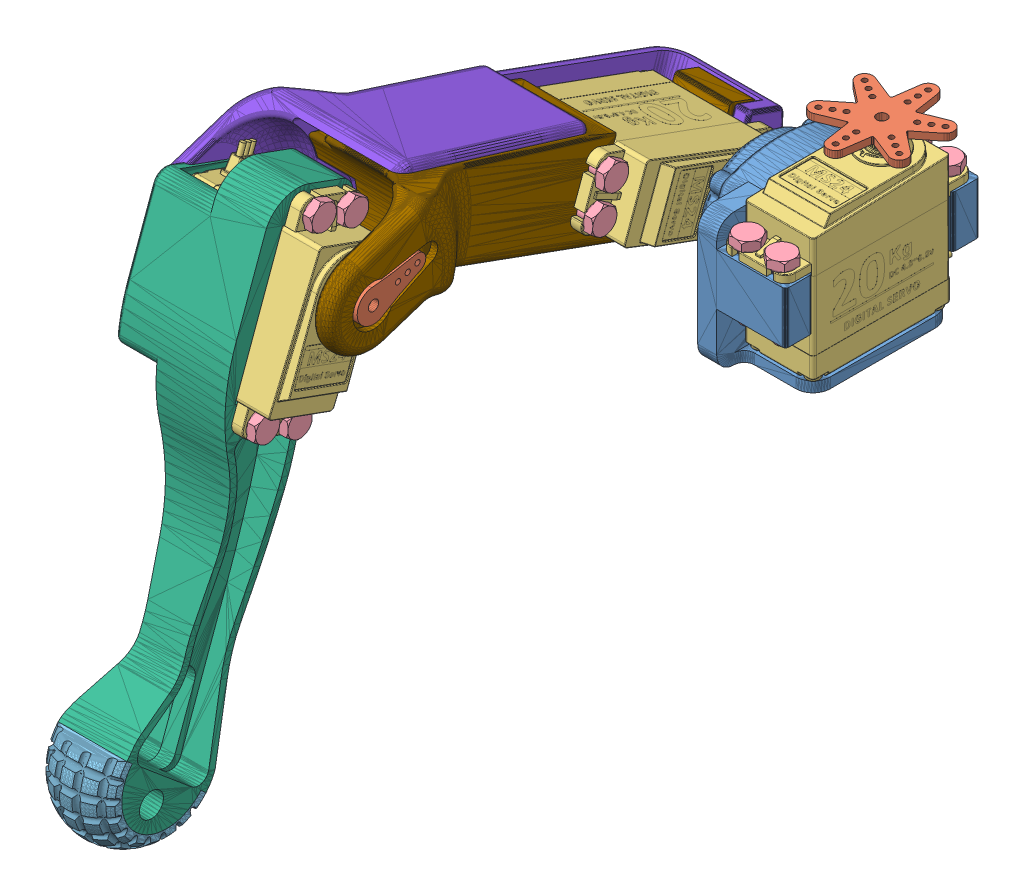
SolidWorks assembly Back Right Leg Assembly, configuration Default. Lengths in mm.
Overall size (104.56 167.25 200.75).
25 component instances, 9 part files, 60 mates.
Components (placement in the parent):
- Right_arm_joint_mg-1: Right_arm_joint_mg [Default] at (24.2858 18.5405 -25.0321) size (37.5 46 56.5)
- Servohorn-1: Servohorn [4 Prong] at (-38.4142 28.7905 -4.7821) x (0 0.715501 0.698611) z (-1 0 0) size (31.8 31.8 2.24)
- Servo Motor-1: Servo Motor [Default] at (-15.7142 38.5405 -14.5321) size (20.1 45.99 55.6)
- Servohorn-2: Servohorn [Default] at (-15.7142 58.9405 -14.5321) x (-0.99999 0 0.00451) z (0 -1 0) size (28.18 31.8 2.24)
- _Hex_Screws-1: _Hex_Screws [H M4x20] at (-20.7142 41.7405 19.4679) x (-0.837169 0 -0.546944) z (-0.546944 0 0.837169) size (7 22.8 8.08)
- _Hex_Screws-2: _Hex_Screws [H M4x20] at (-10.7142 41.7405 -28.5321) x (-0.837169 0 -0.546944) z (-0.546944 0 0.837169) size (7 22.8 8.08)
- _Hex_Screws-3: _Hex_Screws [H M4x20] at (-10.7142 41.7405 19.4679) x (-0.99108 0 -0.133267) z (-0.133267 0 0.99108) size (7 22.8 8.08)
- _Hex_Screws-4: _Hex_Screws [H M4x20] at (-20.7142 41.7405 -28.5321) x (0.837169 0 0.546944) z (0.546944 0 -0.837169) size (7 22.8 8.08)
- _Hex_Screws-20: _Hex_Screws [H M3x16] at (-83.7173 43.6223 71.0537) x (0.992954 0.04053 0.111356) z (-0.118503 0.33961 0.933071) size (5.5 18 6.35)
- _Hex_Screws-21: _Hex_Screws [H M4x20] at (-66.0142 67.1041 99.9555) x (0 0.149128 -0.988818) z (0 0.988818 0.149128) size (7 22.8 8.08)
- _Hex_Screws-22: _Hex_Screws [H M4x20] at (-66.0142 63.6839 90.5585) x (0 -0.837169 0.546944) z (0 -0.546944 -0.837169) size (7 22.8 8.08)
- _Hex_Screws-23: _Hex_Screws [H M4x20] at (-66.0142 21.9989 116.3724) x (0 -0.837169 0.546944) z (0 -0.546944 -0.837169) size (7 22.8 8.08)
- _Hex_Screws-24: _Hex_Screws [H M4x20] at (-66.0142 18.5787 106.9755) x (0 -0.837169 0.546944) z (0 -0.546944 -0.837169) size (7 22.8 8.08)
- _Hex_Screws-25: _Hex_Screws [H M4x20] at (-55.6142 28.7007 -19.6479) x (0 0.663788 -0.747921) z (0 0.747921 0.663788) size (7 22.8 8.08)
- _Hex_Screws-26: _Hex_Screws [H M4x20] at (-55.6142 19.3037 -16.2277) x (0 -0.857577 0.514355) z (0 -0.514355 -0.857577) size (7 22.8 8.08)
- _Hex_Screws-27: _Hex_Screws [H M4x20] at (-55.6142 45.1176 25.4573) x (0 -0.837169 0.546944) z (0 -0.546944 -0.837169) size (7 22.8 8.08)
- _Hex_Screws-28: _Hex_Screws [H M4x20] at (-55.6142 35.7207 28.8775) x (0 -0.837169 0.546944) z (0 -0.546944 -0.837169) size (7 22.8 8.08)
- Servo Motor-4: Servo Motor [Default] at (-69.2142 52.2383 100.0453) x (0 -0.34202 -0.939693) z (0 -0.939693 0.34202) size (20.1 45.99 55.6)
- foot-2: foot [Default] at (-69.2142 -56.7491 139.7664) x (0 -0.642788 -0.766044) z (0 0.766044 -0.642788) size (38.32 20 19.41)
- Left_wrist_mg-1: Left_wrist_mg [Default] at (-39.2142 58.2322 87.2751) x (0 -0.939693 0.34202) z (0 0.34202 0.939693) size (149.99 36.9 30)
- Servohorn-4: Servohorn [1 Prong] at (-48.8142 52.2383 100.0453) x (0 -0.947083 -0.320989) z (-1 0 0) size (9.55 20.65 2.24)
- F625ZZ Ball Bearing-2: F625ZZ Ball Bearing [Default] at (-99.0142 54.8139 92.2998) x (0 0.948801 0.315873) z (1 0 0) size (18 18 5)
- SM_Left_arm_cover-1: SM_Left_arm_cover [Default] at (-59.0142 8.2739 -16.9989) x (0 0.939693 -0.34202) z (0 0.34202 0.939693) size (41.16 45 143.55)
- Left_arm_mg-1: Left_arm_mg [Default] at (-58.8142 15.8365 -11.1347) x (0 0.939693 -0.34202) z (0 0.34202 0.939693) size (38.24 39.8 137.4)
- Servo Motor-5: Servo Motor [Default] at (-58.8142 28.7905 -4.7821) x (0 -0.939693 0.34202) z (0 0.34202 0.939693) size (20.1 45.99 55.6)
Mates (geometry in assembly coordinates):
- Coincident1: coincident anti-aligned: plane of Right_arm_joint_mg-1 through (-40.4142 18.5405 -25.0321) normal (1 0 0); plane of Servohorn-1 through (-40.4142 28.7905 -4.7821) normal (-1 0 0)
- Angle2: planar angle = 0.069813 rad anti-aligned: plane of Right_arm_joint_mg-1 through (24.2858 29.9404 -17.8834) normal (0 0.847204 0.531268); plane of Servohorn-1 through (-40.4142 21.752 -2.4794) normal (0 -0.808081 -0.589071)
- Coincident4: coincident: point of Right_arm_joint_mg-1; line of Servohorn-1 through (-38.4142 28.7905 -4.7821) axis (1 0 0)
- Coincident5: coincident anti-aligned: plane of Right_arm_joint_mg-1 through (-25.7142 18.5405 -25.0321) normal (1 0 0); plane of Servo Motor-1 through (-25.7142 49.5405 -23.5321) normal (-1 0 0)
- Coincident6: coincident anti-aligned: plane of Right_arm_joint_mg-1 through (24.2858 11.0405 -25.0321) normal (0 1 0); plane of Servo Motor-1 through (-15.7142 11.0405 -14.5321) normal (0 -1 0)
- Distance2: distance = 0 mm anti-aligned: plane of Servo Motor-1 through (-25.7142 18.5405 15.4679) normal (0 0 1); plane of Right_arm_joint_mg-1 through (24.2858 18.5405 15.4679) normal (0 0 -1)
- Concentric1: concentric anti-aligned: cylinder of Servo Motor-1 through (-15.7142 52.9405 -14.5321) axis (0 1 0) radius 1.25; line of Servohorn-2 through (-15.7142 58.9405 -14.5321) axis (0 -1 0)
- Coincident8: coincident anti-aligned: plane of Servo Motor-1 through (-15.7142 56.9405 -14.5321) normal (0 1 0); plane of Servohorn-2 through (-15.7142 56.9405 -14.5321) normal (0 -1 0)
- Concentric4: concentric aligned: cylinder of Servo Motor-1 through (-10.7142 32.1765 19.4679) axis (0 1 0) radius 2.25; cylinder of _Hex_Screws-3 through (-10.7142 21.7405 19.4679) axis (0 1 0) radius 2
- Coincident35: coincident anti-aligned: plane of Servo Motor-1 through (-15.7142 41.7405 -14.5321) normal (0 1 0); plane of _Hex_Screws-3 through (-10.7142 41.7405 19.4679) normal (0 -1 0)
- Concentric5: concentric aligned: cylinder of Servo Motor-1 through (-20.7142 32.1765 19.4679) axis (0 1 0) radius 2.25; cylinder of _Hex_Screws-1 through (-20.7142 21.7405 19.4679) axis (0 1 0) radius 2
- Coincident36: coincident aligned: plane of _Hex_Screws-1 through (-20.7142 44.5405 19.4679) normal (0 1 0); plane of _Hex_Screws-3 through (-10.7142 44.5405 19.4679) normal (0 1 0)
- Concentric6: concentric aligned: cylinder of Servo Motor-1 through (-20.7142 32.1765 -28.5321) axis (0 1 0) radius 2.25; cylinder of _Hex_Screws-4 through (-20.7142 21.7405 -28.5321) axis (0 1 0) radius 2
- Coincident37: coincident anti-aligned: plane of Servo Motor-1 through (-15.7142 41.7405 -14.5321) normal (0 1 0); plane of _Hex_Screws-4 through (-20.7142 41.7405 -28.5321) normal (0 -1 0)
- Concentric7: concentric aligned: cylinder of Servo Motor-1 through (-10.7142 32.1765 -28.5321) axis (0 1 0) radius 2.25; cylinder of _Hex_Screws-2 through (-10.7142 21.7405 -28.5321) axis (0 1 0) radius 2
- Coincident38: coincident anti-aligned: plane of Servo Motor-1 through (-15.7142 41.7405 -14.5321) normal (0 1 0); plane of _Hex_Screws-2 through (-10.7142 41.7405 -28.5321) normal (0 -1 0)
- Coincident50: coincident anti-aligned: plane of Left_arm_mg-1 through (-58.8142 15.8365 -11.1347) normal (1 0 0); plane of Servo Motor-5 through (-58.8142 29.5678 23.6678) normal (-1 0 0)
- Angle5: planar angle = 0.069813 rad aligned: line of Left_arm_mg-1 through (-48.8142 60.1418 84.6186) axis (0 -0.180422 0.983589); line of Servohorn-4 through (-48.8142 57.5916 94.928) axis (0 -0.111371 0.993779)
- Coincident51: coincident anti-aligned: plane of Servo Motor-4 through (-96.7142 65.1665 106.0348) normal (0 0.34202 0.939693); plane of Left_wrist_mg-1 through (-39.2142 65.0726 106.069) normal (0 -0.34202 -0.939693)
- Coincident52: coincident: point of foot-2; line of Left_wrist_mg-1 through (-89.2142 -66.7075 148.1228) axis (0 0.687865 0.725839)
- Coincident53: coincident anti-aligned: plane of SM_Left_arm_cover-1 through (-59.0142 38.9729 67.346) normal (0 -0.34202 -0.939693); plane of Left_arm_mg-1 through (-58.8142 43.7662 65.6014) normal (0 0.34202 0.939693)
- Coincident54: coincident anti-aligned: plane of Servo Motor-4 through (-50.8142 52.2383 100.0453) normal (1 0 0); plane of Servohorn-4 through (-50.8142 52.2383 100.0453) normal (-1 0 0)
- Coincident55: coincident aligned: plane of foot-2 through (-89.2142 -56.7491 139.7664) normal (-1 0 0); plane of Left_wrist_mg-1 through (-89.2142 58.2322 87.2751) normal (-1 0 0)
- Coincident56: coincident anti-aligned: plane of SM_Left_arm_cover-1 through (-59.0142 15.3535 -19.5757) normal (0 -0.939693 0.34202); plane of Left_arm_mg-1 through (-58.8142 18.1228 -11.9669) normal (0 0.939693 -0.34202)
- Concentric8: concentric aligned: cylinder of Servo Motor-4 through (-54.8142 52.2383 100.0453) axis (1 0 0) radius 1.25; line of Servohorn-4 through (-48.8142 52.2383 100.0453) axis (1 0 0)
- Concentric9: concentric aligned: cylinder of _Hex_Screws-28 through (-75.6142 35.7207 28.8775) axis (1 0 0) radius 2; cylinder of Servo Motor-5 through (-65.1781 35.7207 28.8775) axis (1 0 0) radius 2.25
- Coincident57: coincident anti-aligned: plane of Servohorn-4 through (-50.8142 52.2383 100.0453) normal (-1 0 0); plane of Left_arm_mg-1 through (-50.8142 15.8365 -11.1347) normal (1 0 0)
- Concentric10: concentric aligned: cylinder of _Hex_Screws-27 through (-75.6142 45.1176 25.4573) axis (1 0 0) radius 2; cylinder of Servo Motor-5 through (-65.1781 45.1176 25.4573) axis (1 0 0) radius 2.25
- Coincident58: coincident anti-aligned: plane of Servo Motor-4 through (-69.2142 23.7885 100.8226) normal (-1 0 0); plane of Left_wrist_mg-1 through (-69.2142 58.2322 87.2751) normal (1 0 0)
- Coincident59: coincident anti-aligned: plane of F625ZZ Ball Bearing-2 through (-100.0142 49.7599 107.4806) normal (-1 0 0); plane of SM_Left_arm_cover-1 through (-100.0142 8.2739 -16.9989) normal (1 0 0)
- Coincident60: coincident anti-aligned: plane of SM_Left_arm_cover-1 through (-63.8142 8.2739 -16.9989) normal (-1 0 0); plane of Left_arm_mg-1 through (-63.8142 15.8365 -11.1347) normal (1 0 0)
- Coincident61: coincident anti-aligned: plane of Left_arm_mg-1 through (-58.8142 15.8365 -11.1347) normal (0 0.939693 -0.34202); plane of Servo Motor-5 through (-47.8142 29.3121 25.8892) normal (0 -0.939693 0.34202)
- Coincident62: coincident anti-aligned: plane of Left_arm_mg-1 through (-58.8142 29.6884 26.9228) normal (0 -0.34202 -0.939693); plane of Servo Motor-5 through (-86.3142 48.5292 20.0653) normal (0 0.34202 0.939693)
- Coincident63: coincident aligned: line of Servohorn-4 through (-48.8142 52.2383 100.0453) axis (1 0 0); line of Left_arm_mg-1 through (-50.8142 52.2383 100.0453) axis (1 0 0)
- Coincident64: coincident anti-aligned: plane of foot-2 through (-69.2142 -56.7491 139.7664) normal (0 0.766044 -0.642788); plane of Left_wrist_mg-1 through (-39.2142 -35.0884 165.5805) normal (0 -0.766044 0.642788)
- Coincident65: coincident anti-aligned: plane of Servo Motor-4 through (-89.2142 65.0555 106.022) normal (0 0.939693 -0.34202); plane of Left_wrist_mg-1 through (-39.2142 58.2322 87.2751) normal (0 -0.939693 0.34202)
- Concentric11: concentric aligned: cylinder of _Hex_Screws-23 through (-86.0142 21.9989 116.3724) axis (1 0 0) radius 2; cylinder of Servo Motor-4 through (-75.5781 21.9989 116.3724) axis (1 0 0) radius 2.25
- Concentric12: concentric aligned: cylinder of _Hex_Screws-26 through (-75.6142 19.3037 -16.2277) axis (1 0 0) radius 2; cylinder of Servo Motor-5 through (-65.1781 19.3037 -16.2277) axis (1 0 0) radius 2.25
- Coincident66: coincident anti-aligned: plane of _Hex_Screws-24 through (-66.0142 18.5787 106.9755) normal (-1 0 0); plane of Servo Motor-4 through (-66.0142 52.2383 100.0453) normal (1 0 0)
- Concentric13: concentric aligned: cylinder of _Hex_Screws-24 through (-86.0142 18.5787 106.9755) axis (1 0 0) radius 2; cylinder of Servo Motor-4 through (-75.5781 18.5787 106.9755) axis (1 0 0) radius 2.25
- Coincident67: coincident anti-aligned: plane of _Hex_Screws-28 through (-55.6142 35.7207 28.8775) normal (-1 0 0); plane of Servo Motor-5 through (-55.6142 28.7905 -4.7821) normal (1 0 0)
- Coincident68: coincident anti-aligned: plane of _Hex_Screws-23 through (-66.0142 21.9989 116.3724) normal (-1 0 0); plane of Servo Motor-4 through (-66.0142 52.2383 100.0453) normal (1 0 0)
- Coincident69: coincident anti-aligned: plane of _Hex_Screws-25 through (-55.6142 28.7007 -19.6479) normal (-1 0 0); plane of Servo Motor-5 through (-55.6142 28.7905 -4.7821) normal (1 0 0)
- Angle6: planar angle = 1.570796 rad anti-aligned: plane of Servo Motor-4 through (-58.2142 21.5671 100.5669) normal (0 -0.34202 -0.939693); plane of Left_arm_mg-1 through (-58.8142 11.1381 -9.4246) normal (0 -0.939693 0.34202)
- Concentric14: concentric aligned: cylinder of _Hex_Screws-22 through (-86.0142 63.6839 90.5585) axis (1 0 0) radius 2; cylinder of Servo Motor-4 through (-75.5781 63.6839 90.5585) axis (1 0 0) radius 2.25
- Coincident70: coincident anti-aligned: plane of _Hex_Screws-27 through (-55.6142 45.1176 25.4573) normal (-1 0 0); plane of Servo Motor-5 through (-55.6142 28.7905 -4.7821) normal (1 0 0)
- Concentric15: concentric aligned: cylinder of _Hex_Screws-25 through (-75.6142 28.7007 -19.6479) axis (1 0 0) radius 2; cylinder of Servo Motor-5 through (-65.1781 28.7007 -19.6479) axis (1 0 0) radius 2.25
- Coincident71: coincident anti-aligned: plane of _Hex_Screws-26 through (-55.6142 19.3037 -16.2277) normal (-1 0 0); plane of Servo Motor-5 through (-55.6142 28.7905 -4.7821) normal (1 0 0)
- Concentric16: concentric aligned: cylinder of _Hex_Screws-21 through (-86.0142 67.1041 99.9555) axis (1 0 0) radius 2; cylinder of Servo Motor-4 through (-75.5781 67.1041 99.9555) axis (1 0 0) radius 2.25
- Coincident72: coincident anti-aligned: plane of _Hex_Screws-20 through (-83.7173 43.6223 71.0537) normal (0 0.939693 -0.34202); plane of Left_arm_mg-1 through (-58.8142 13.9572 -10.4507) normal (0 -0.939693 0.34202)
- Coincident73: coincident anti-aligned: plane of _Hex_Screws-22 through (-66.0142 63.6839 90.5585) normal (-1 0 0); plane of Servo Motor-4 through (-66.0142 52.2383 100.0453) normal (1 0 0)
- Tangent1: tangent anti-aligned: cylinder of F625ZZ Ball Bearing-2 through (-102.0142 52.2869 99.8902) axis (-1 0 0) radius 8; plane of SM_Left_arm_cover-1 through (-59.0142 59.281 103.8533) normal (0 -0.914236 -0.405181)
- Tangent2: tangent anti-aligned: cylinder of _Hex_Screws-20 through (-83.7173 58.6574 65.5814) axis (0 -0.939693 0.34202) radius 1.5; plane of Left_arm_mg-1 through (-93.0304 17.3773 -6.9017) normal (-0.991445 0.044643 0.122657)
- Tangent3: tangent anti-aligned: cylinder of F625ZZ Ball Bearing-2 through (-102.0142 52.2869 99.8902) axis (-1 0 0) radius 8; plane of SM_Left_arm_cover-1 through (-59.0142 53.9278 92.0469) normal (0 -0.148446 0.988921)
- Tangent4: tangent anti-aligned: cylinder of _Hex_Screws-20 through (-83.7173 58.6574 65.5814) axis (0 -0.939693 0.34202) radius 1.5; plane of Left_arm_mg-1 through (-47.8174 44.4025 67.3497) normal (-0.130537 -0.339094 -0.931652)
- Concentric17: concentric aligned: line of Servohorn-1 through (-38.4142 28.7905 -4.7821) axis (1 0 0); cylinder of Servo Motor-5 through (-44.4142 28.7905 -4.7821) axis (1 0 0) radius 1.25
- Concentric18: concentric aligned: cylinder of _Hex_Screws-21 through (-86.0142 67.1041 99.9555) axis (1 0 0) radius 2; cylinder of Servo Motor-4 through (-75.5781 67.1041 99.9555) axis (1 0 0) radius 2.25
- Coincident74: coincident anti-aligned: plane of _Hex_Screws-21 through (-66.0142 67.1041 99.9555) normal (-1 0 0); plane of Servo Motor-4 through (-66.0142 52.2383 100.0453) normal (1 0 0)
- Coincident75: coincident anti-aligned: plane of Servohorn-1 through (-40.4142 28.7905 -4.7821) normal (-1 0 0); plane of Servo Motor-5 through (-40.4142 28.7905 -4.7821) normal (1 0 0)
- Angle7: planar angle = 0.349066 rad aligned: plane of Right_arm_joint_mg-1 through (24.2858 18.5405 -33.0321) normal (0 0 -1); plane of Left_arm_mg-1 through (-58.8142 13.1004 -18.6523) normal (0 -0.34202 -0.939693)
